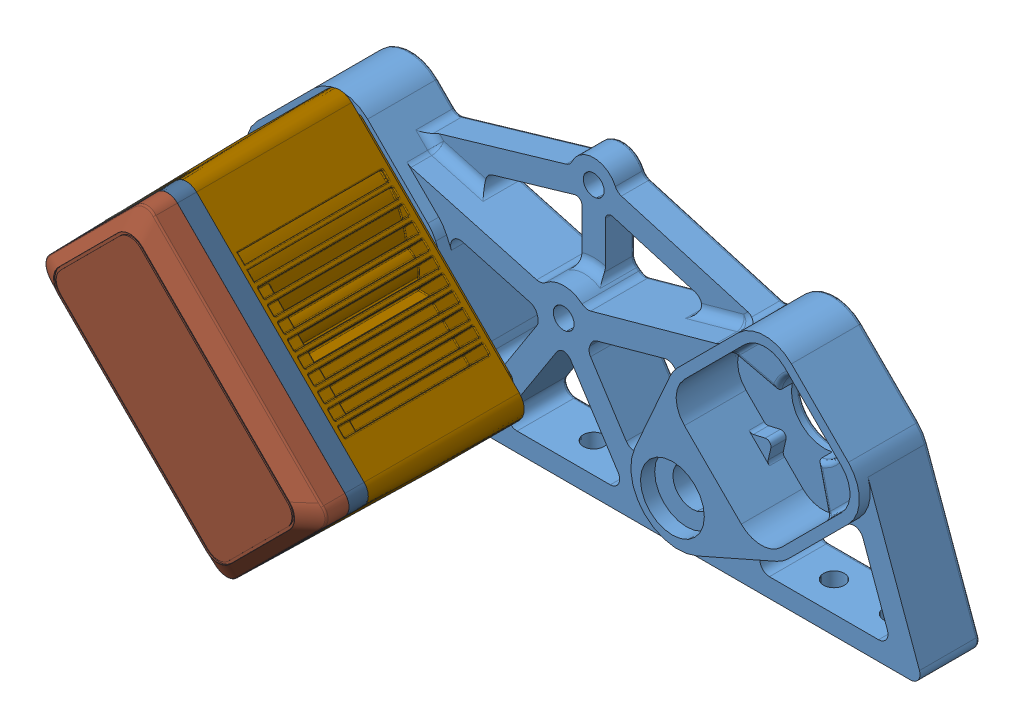
SolidWorks assembly inner_bracket_testing, configuration Default. Lengths in mm.
Overall size (150.69 67.96 59.91).
22 component instances, 13 part files, 3 mates.
Components (placement in the parent):
- chassis_inner_bracket-1: chassis_inner_bracket [Default] at (1.5109 76.0814 146.2919) size (150.69 55.8 15.04)
- V5 Smart Motor (276-4840) no cap-1: V5 Smart Motor (276-4840) no cap [Default] at (54.9412 103.0221 178.4919) x (-0.707107 0.707107 0) z (0 0 -1) size (59.01 35.33 59.91)
  - V5 Smart Motor (276-4840).step-1: V5 Smart Motor (276-4840).step [Default] at origin size (59.01 35.33 59.91)
    - 276-4840-900 Rev6_Instruction.step-1: 276-4840-900 Rev6_Instruction.step [Default] at (-14.3 0 -17.2) size (52.79 15.94 38.15)
      - 276-4840-901 Rev6.step-1: 276-4840-901 Rev6.step [Default] at (10.75 -10.05 17.8) x (-1 0 0) z (0 0 1) size (49.9 1.6 38.15)
      - 276-4840-902 Rev2.step-1: 276-4840-902 Rev2.step [Default] at (31.25 -9.25 6.2) x (0 0 -1) z (0 -1 0) size (10.35 11.39 15.94)
      - 276-4840-022 Rev4.step-1: 276-4840-022 Rev4.step [Default] at (31.25 -9.25 6.2) x (0 0 -1) z (1 0 0) size (10.26 9.1 5.51)
    - 276-4840-110 Rev10_Instruction.step-1: 276-4840-110 Rev10_Instruction.step [Default] at (12.7 0 14.7) size (35.33 35.33 31.1)
      - 276-4840-061 Rev7_Ring_Gear_Fixed01 .6 Rev3.step-1: 276-4840-061 Rev7_Ring_Gear_Fixed01 .6 Rev3.step [Default] at origin size (28.79 28.39 24.6)
      - 276-4840-018 Rev6.step-1: 276-4840-018 Rev6.step [Default] at (0 0 6.7) x (-0.483174 0.875524 0) z (0 0 1) size (26 26 12.3)
      - 276-4840-059 Rev2.step-1: 276-4840-059 Rev2.step [Default] at (0 0 10.3) size (28.4 28.4 8.5)
      - 276-4840-062 Rev1.step-1: 276-4840-062 Rev1.step [Default] at (-12.1353 8.8168 12.3) x (0.956835 -0.290632 0) z (-0.290632 -0.956835 0) size (3.2 6.56 3.2)
      - 276-4840-062 Rev1.step-2: 276-4840-062 Rev1.step [Default] at (12.1353 8.8168 12.3) x (0.978427 0.206591 0) z (0.206591 -0.978427 0) size (3.2 6.56 3.2)
      - 276-4840-062 Rev1.step-3: 276-4840-062 Rev1.step [Default] at (-12.1353 -8.8168 12.3) x (0.72563 0.688086 0) z (0.688086 -0.72563 0) size (3.2 6.56 3.2)
    - 276-4840-001 Rev38.step-1: 276-4840-001 Rev38.step [Default] at origin size (57.3 33 46.9)
    - 276-4840-005 Rev27.step-1: 276-4840-005 Rev27.step [Default] at (0 0 -17.95) size (56.17 31.87 12.9)
    - 276-4840-004 Rev16.step-1: 276-4840-004 Rev16.step [Default] at (0 0 -19.2) size (56.01 31.71 9.21)
    - 276-4840-009 Rev3.step-1: 276-4840-009 Rev3.step [Default] at (25.45 13.5 15.7) x (0.19987 -0.979823 0) z (-0.979823 -0.19987 0) size (3.4 41.31 4.34)
    - 276-4840-009 Rev3.step-2: 276-4840-009 Rev3.step [Default] at (-25.45 -13.5 15.7) x (-0.998855 0.047836 0) z (0.047836 0.998855 0) size (3.4 41.31 4.34)
    - 276-4840-009 Rev3.step-3: 276-4840-009 Rev3.step [Default] at (25.45 -13.5 15.7) x (-0.975374 0.220559 0) z (0.220559 0.975374 0) size (3.4 41.31 4.34)
    - 276-4840-009 Rev3.step-4: 276-4840-009 Rev3.step [Default] at (-25.45 13.5 15.7) x (-0.922256 0.38658 0) z (0.38658 0.922256 0) size (3.4 41.31 4.34)
    - 276-4840-025 Rev19.step-1: 276-4840-025 Rev19.step [Default] at (12.7 0 -22.63) x (-0.993315 0.115437 0) z (0 0 1) size (14.82 14.83 35.18)
Mates (geometry in assembly coordinates):
- Coincident1: coincident anti-aligned: plane of chassis_inner_bracket-1 through (1.5109 76.0814 161.2919) normal (0 0 1); plane of V5 Smart Motor (276-4840) no cap-1/V5 Smart Motor (276-4840).step-1/276-4840-001 Rev38.step-1 through (81.7759 94.4308 161.2919) normal (0 0 -1)
- Parallel1: parallel anti-aligned: line of chassis_inner_bracket-1 through (39.9505 130.0336 161.2919) axis (-0.707107 -0.707107 0); line of V5 Smart Motor (276-4840) no cap-1/V5 Smart Motor (276-4840).step-1/276-4840-001 Rev38.step-1 through (25.5609 114.1591 162.2919) axis (0.707107 0.707107 0)
- Concentric1: concentric aligned: circle of chassis_inner_bracket-1; circle of V5 Smart Motor (276-4840) no cap-1/V5 Smart Motor (276-4840).step-1/276-4840-110 Rev10_Instruction.step-1/276-4840-059 Rev2.step-1
